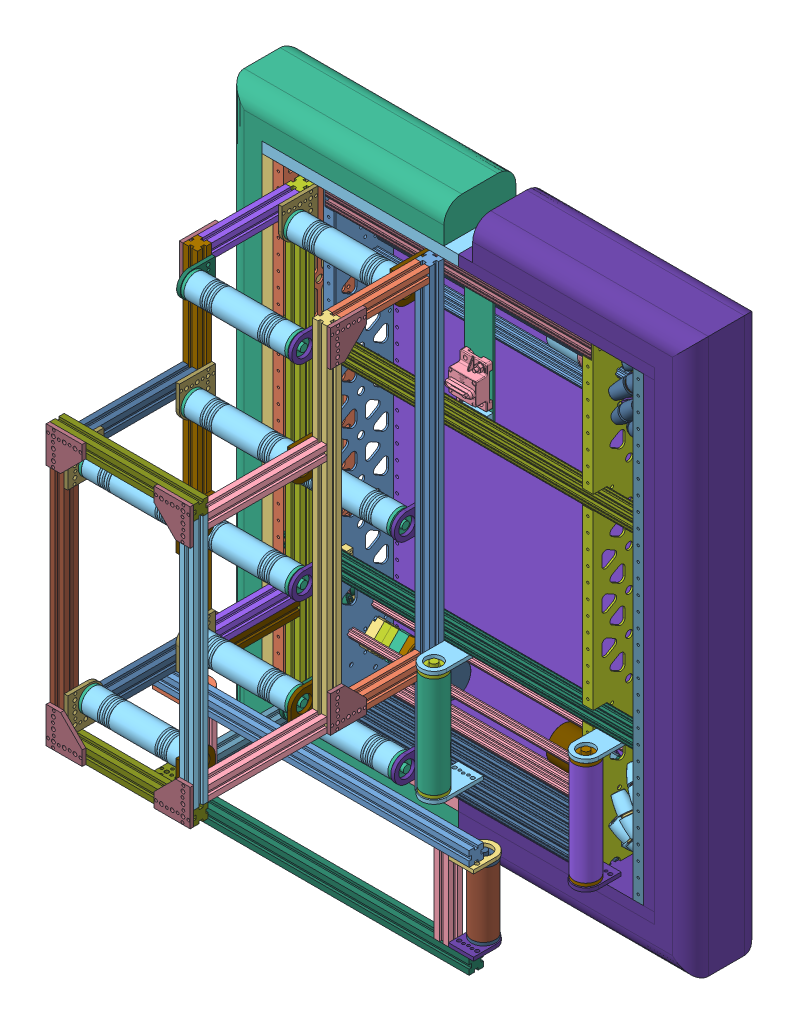
SolidWorks assembly Robot 2020, configuration Default. Lengths in mm.
Overall size (819.15 977.9 619.08).
518 component instances, 131 part files, 0 mates.
Components (placement in the parent):
- Copy of Fame 2020-1: Copy of Fame 2020 [Default] at origin size (819.15 977.9 171.99)
  - Inner plate v12(Mirror)^Copy of Fame 2020-1: Inner plate v12(Mirror)^Copy of Fame 2020 [Default] at (-212.725 0 58.7875) x (0 1 0) z (0 0 -1) size (812.8 19.05 127) (virtual)
    - Inner plate v12(Mirror)-0^Inner plate v12(Mirror)_Copy of Fame 2020-1: Inner plate v12(Mirror)-0^Inner plate v12(Mirror)_Copy of Fame 2020 [Default] at origin size (812.8 19.05 127) (virtual)
  - Outer plate v11(Mirror)^Copy of Fame 2020-1: Outer plate v11(Mirror)^Copy of Fame 2020 [Default] at (-333.375 0 58.7875) x (0 -1 0) z (0 0 -1) size (812.8 19.05 127) (virtual)
    - Outer plate v11(Mirror)-1^Outer plate v11(Mirror)_Copy of Fame 2020-1: Outer plate v11(Mirror)-1^Outer plate v11(Mirror)_Copy of Fame 2020 [Default] at origin size (812.8 19.05 127) (virtual)
  - Bumper Assembly v4(Mirror)^Copy of Fame 2020-1: Bumper Assembly v4(Mirror)^Copy of Fame 2020 [Default] at (-327.025 0.0665 58.7875) x (-1 0 0) z (0 0 -1) size (409.58 977.9 127) (virtual)
    - Bumper Assembly v4(Mirror)-2^Bumper Assembly v4(Mirror)_Copy of Fame 2020-1: Bumper Assembly v4(Mirror)-2^Bumper Assembly v4(Mirror)_Copy of Fame 2020 [Default] at origin size (19.05 812.8 127) (virtual)
    - Bumper Assembly v4(Mirror)-3^Bumper Assembly v4(Mirror)_Copy of Fame 2020-1: Bumper Assembly v4(Mirror)-3^Bumper Assembly v4(Mirror)_Copy of Fame 2020 [Default] at origin size (346.08 19.05 127) (virtual)
    - Bumper Assembly v4(Mirror)-4^Bumper Assembly v4(Mirror)_Copy of Fame 2020-1: Bumper Assembly v4(Mirror)-4^Bumper Assembly v4(Mirror)_Copy of Fame 2020 [Default] at origin size (346.08 19.05 127) (virtual)
    - Bumper Assembly v4(Mirror)-5^Bumper Assembly v4(Mirror)_Copy of Fame 2020-1: Bumper Assembly v4(Mirror)-5^Bumper Assembly v4(Mirror)_Copy of Fame 2020 [Default] at origin size (409.58 977.9 127) (virtual)
  - NEO Gearbox 2-stage Custom^Copy of Fame 2020-1: NEO Gearbox 2-stage Custom^Copy of Fame 2020 [Default] at (0 0 425) size (164.9 90.53 90.53) (virtual)
    - VersaPlanetary_4_1_Gear_Kit_217-2818^NEO Gearbox 2-stage Custom_Copy of Fame 2020-1: VersaPlanetary_4_1_Gear_Kit_217-2818^NEO Gearbox 2-stage Custom_Copy of Fame 2020 [Default] at (-15.25 22.225 0) x (0 -0.707107 0.707107) z (-1 0 0) size (35.49 35.49 17.4) (virtual)
      - 217-2725-001 Rev1_24t Sun^VersaPlanetary_4_1_Gear_Kit_217-2818_NEO Gearbox 2-stage Custom_Copy of Fame 2020-1: 217-2725-001 Rev1_24t Sun^VersaPlanetary_4_1_Gear_Kit_217-2818_NEO Gearbox 2-stage Custom_Copy of Fame 2020 [Default] at (-36.69 -517.1337 -209.675) x (0.707107 0.707107 0) z (0 0 1) size (14.4 14.45 12.7) (virtual)
      - 217-2725-002 Rev1_24t Planet^VersaPlanetary_4_1_Gear_Kit_217-2818_NEO Gearbox 2-stage Custom_Copy of Fame 2020-1: 217-2725-002 Rev1_24t Planet^VersaPlanetary_4_1_Gear_Kit_217-2818_NEO Gearbox 2-stage Custom_Copy of Fame 2020 [Default] at (-45.2382 -525.6819 -212.025) x (-0.793353 0.608761 0) z (0 0 -1) size (13.12 13.1 8) (virtual)
      - 217-2724-002 Rev1^VersaPlanetary_4_1_Gear_Kit_217-2818_NEO Gearbox 2-stage Custom_Copy of Fame 2020-1: 217-2724-002 Rev1^VersaPlanetary_4_1_Gear_Kit_217-2818_NEO Gearbox 2-stage Custom_Copy of Fame 2020 [Default] at (-36.69 -517.1337 -218.375) x (1 0 0) z (0 0 -1) size (34.7 34.7 4.7) (virtual)
      - 217-2625-010 Rev1^VersaPlanetary_4_1_Gear_Kit_217-2818_NEO Gearbox 2-stage Custom_Copy of Fame 2020-1: 217-2625-010 Rev1^VersaPlanetary_4_1_Gear_Kit_217-2818_NEO Gearbox 2-stage Custom_Copy of Fame 2020 [Default] at (-45.2382 -525.6819 -214.725) x (0.854322 0.519745 0) z (0 0 1) size (4 4 12) (virtual)
      - 217-2725-002 Rev1_24t Planet^VersaPlanetary_4_1_Gear_Kit_217-2818_NEO Gearbox 2-stage Custom_Copy of Fame 2020-2: 217-2725-002 Rev1_24t Planet^VersaPlanetary_4_1_Gear_Kit_217-2818_NEO Gearbox 2-stage Custom_Copy of Fame 2020 [Default] at (-28.1418 -525.6819 -212.025) x (-0.608761 -0.793353 0) z (0 0 -1) size (13.12 13.1 8) (virtual)
      - 217-2725-002 Rev1_24t Planet^VersaPlanetary_4_1_Gear_Kit_217-2818_NEO Gearbox 2-stage Custom_Copy of Fame 2020-3: 217-2725-002 Rev1_24t Planet^VersaPlanetary_4_1_Gear_Kit_217-2818_NEO Gearbox 2-stage Custom_Copy of Fame 2020 [Default] at (-28.1418 -508.5855 -212.025) x (0.793353 -0.608761 0) z (0 0 -1) size (13.12 13.1 8) (virtual)
      - 217-2725-002 Rev1_24t Planet^VersaPlanetary_4_1_Gear_Kit_217-2818_NEO Gearbox 2-stage Custom_Copy of Fame 2020-4: 217-2725-002 Rev1_24t Planet^VersaPlanetary_4_1_Gear_Kit_217-2818_NEO Gearbox 2-stage Custom_Copy of Fame 2020 [Default] at (-45.2382 -508.5855 -212.025) x (0.608761 0.793353 0) z (0 0 -1) size (13.12 13.1 8) (virtual)
      - 217-2625-010 Rev1^VersaPlanetary_4_1_Gear_Kit_217-2818_NEO Gearbox 2-stage Custom_Copy of Fame 2020-2: 217-2625-010 Rev1^VersaPlanetary_4_1_Gear_Kit_217-2818_NEO Gearbox 2-stage Custom_Copy of Fame 2020 [Default] at (-28.1418 -525.6819 -214.725) x (-0.519745 0.854322 0) z (0 0 1) size (4 4 12) (virtual)
      - 217-2625-010 Rev1^VersaPlanetary_4_1_Gear_Kit_217-2818_NEO Gearbox 2-stage Custom_Copy of Fame 2020-3: 217-2625-010 Rev1^VersaPlanetary_4_1_Gear_Kit_217-2818_NEO Gearbox 2-stage Custom_Copy of Fame 2020 [Default] at (-28.1418 -508.5855 -214.725) x (-0.854322 -0.519745 0) z (0 0 1) size (4 4 12) (virtual)
      - 217-2625-010 Rev1^VersaPlanetary_4_1_Gear_Kit_217-2818_NEO Gearbox 2-stage Custom_Copy of Fame 2020-4: 217-2625-010 Rev1^VersaPlanetary_4_1_Gear_Kit_217-2818_NEO Gearbox 2-stage Custom_Copy of Fame 2020 [Default] at (-45.2382 -508.5855 -214.725) x (0.519745 -0.854322 0) z (0 0 1) size (4 4 12) (virtual)
    - 217-2625-026 Rev1^NEO Gearbox 2-stage Custom_Copy of Fame 2020-1: 217-2625-026 Rev1^NEO Gearbox 2-stage Custom_Copy of Fame 2020 [Default] at (211.875 -317.5 -391.6125) x (0 -0.707107 0.707107) z (-1 0 0) size (44.45 42 18.12) (virtual)
    - 217-2742-001 Rev4^NEO Gearbox 2-stage Custom_Copy of Fame 2020-1: 217-2742-001 Rev4^NEO Gearbox 2-stage Custom_Copy of Fame 2020 [Default] at (218.5752 -317.5 -391.6125) x (1 0 0) z (0 0.63857 0.769564) size (7 28 28) (virtual)
    - 217-2742-001 Rev4^NEO Gearbox 2-stage Custom_Copy of Fame 2020-2: 217-2742-001 Rev4^NEO Gearbox 2-stage Custom_Copy of Fame 2020 [Default] at (226.5752 -317.5 -391.6125) x (1 0 0) z (0 0.707107 0.707107) size (7 28 28) (virtual)
    - 217-2625-017 Rev1_9714K61^NEO Gearbox 2-stage Custom_Copy of Fame 2020-1: 217-2625-017 Rev1_9714K61^NEO Gearbox 2-stage Custom_Copy of Fame 2020 [Default] at (225.795 -317.6887 -391.9075) x (0 0.983393 0.181491) z (0 -0.181491 0.983393) size (28.51 4.98 27.43) (virtual)
    - 217-2625-025 Rev1^NEO Gearbox 2-stage Custom_Copy of Fame 2020-1: 217-2625-025 Rev1^NEO Gearbox 2-stage Custom_Copy of Fame 2020 [Default] at (182.475 -317.5 -391.6125) x (0 -0.707107 0.707107) z (-1 0 0) size (44.45 42 18) (virtual)
    - 217-2816-001 Rev1^NEO Gearbox 2-stage Custom_Copy of Fame 2020-1: 217-2816-001 Rev1^NEO Gearbox 2-stage Custom_Copy of Fame 2020 [Default] at (212.025 -317.5 -391.6125) x (0 -0.707107 0.707107) z (1 0 0) size (42 42 14.5) (virtual)
    - 217-2816-001 Rev1^NEO Gearbox 2-stage Custom_Copy of Fame 2020-2: 217-2816-001 Rev1^NEO Gearbox 2-stage Custom_Copy of Fame 2020 [Default] at (199.325 -317.5 -391.6125) x (0 -0.707107 0.707107) z (1 0 0) size (42 42 14.5) (virtual)
    - 217-4649-001 Rev1^NEO Gearbox 2-stage Custom_Copy of Fame 2020-1: 217-4649-001 Rev1^NEO Gearbox 2-stage Custom_Copy of Fame 2020 [Default] at (185.629 -317.5 -391.6125) x (0 -0.707107 0.707107) z (1 0 0) size (18 18 13) (virtual)
    - VersaPlanetary_CIM_Adapter_217-4018^NEO Gearbox 2-stage Custom_Copy of Fame 2020-1: VersaPlanetary_CIM_Adapter_217-4018^NEO Gearbox 2-stage Custom_Copy of Fame 2020 [Default] at (165.15 -317.5 -391.6125) x (0 -0.707107 0.707107) z (0 0.707107 0.707107) size (64.01 21.55 64.01) (virtual)
    - NEO Motor REV-21-1650^NEO Gearbox 2-stage Custom_Copy of Fame 2020-1: NEO Motor REV-21-1650^NEO Gearbox 2-stage Custom_Copy of Fame 2020 [Default] at (153.625 -317.5 -391.6125) x (0 -0.707107 -0.707107) z (1 0 0) size (61.14 61.02 93.25) (virtual)
    - 3_1 Output Shaft Custom^NEO Gearbox 2-stage Custom_Copy of Fame 2020-1: 3_1 Output Shaft Custom^NEO Gearbox 2-stage Custom_Copy of Fame 2020 [Default] at (211.3752 -317.5 -391.6125) x (1 0 0) z (0 0.707107 0.707107) size (48.9 34.7 34.7) (virtual)
  - Left Wheel Assembly^Copy of Fame 2020-1: Left Wheel Assembly^Copy of Fame 2020 [Default] at (500 0 0) size (65.82 166.11 165.01) (virtual)
    - 6_Mecanum_Wheel_Left_217-2799^Left Wheel Assembly_Copy of Fame 2020-1: 6_Mecanum_Wheel_Left_217-2799^Left Wheel Assembly_Copy of Fame 2020 [Default] x (0 0 1) z (-1 0 0) size (165.01 166.11 65.82) (virtual)
      - 217-2799-001 Rev1^6_Mecanum_Wheel_Left_217-2799_Left Wheel Assembly_Copy of Fame 2020-1: 217-2799-001 Rev1^6_Mecanum_Wheel_Left_217-2799_Left Wheel Assembly_Copy of Fame 2020 [Default] at (33.3875 -317.5 234.0098) x (0.707107 0.707107 0) z (0 0 1) size (95.78 100.46 28.55) (virtual)
      - 217-2799-001 Rev1^6_Mecanum_Wheel_Left_217-2799_Left Wheel Assembly_Copy of Fame 2020-2: 217-2799-001 Rev1^6_Mecanum_Wheel_Left_217-2799_Left Wheel Assembly_Copy of Fame 2020 [Default] at (33.3875 -317.5 221.3098) x (-0.987688 -0.156434 0) z (0 0 -1) size (95.78 100.46 28.55) (virtual)
      - 217-2799-002 Rev1^6_Mecanum_Wheel_Left_217-2799_Left Wheel Assembly_Copy of Fame 2020-1: 217-2799-002 Rev1^6_Mecanum_Wheel_Left_217-2799_Left Wheel Assembly_Copy of Fame 2020 [Default] at (4.057 -346.8305 227.6598) x (-0.707107 0.707107 0) z (-0.707107 -0.707107 0) size (26.84 25.39 30.1) (virtual)
      - 217-2586-003 Rev2^6_Mecanum_Wheel_Left_217-2799_Left Wheel Assembly_Copy of Fame 2020-1: 217-2586-003 Rev2^6_Mecanum_Wheel_Left_217-2799_Left Wheel Assembly_Copy of Fame 2020 [Default] at (-13.4676 -358.6894 223.6536) x (0.41944 0.854155 0.30739) z (-0.757674 0.142894 0.636798) size (19.46 28.57 19.46) (virtual)
      - 217-2586-003 Rev2^6_Mecanum_Wheel_Left_217-2799_Left Wheel Assembly_Copy of Fame 2020-2: 217-2586-003 Rev2^6_Mecanum_Wheel_Left_217-2799_Left Wheel Assembly_Copy of Fame 2020 [Default] at (-7.8019 -364.3551 231.666) x (0.847342 0.451134 -0.280161) z (0.17892 -0.739241 -0.649238) size (19.46 28.57 19.46) (virtual)
      - 217-2586-004 Rev1^6_Mecanum_Wheel_Left_217-2799_Left Wheel Assembly_Copy of Fame 2020-1: 217-2586-004 Rev1^6_Mecanum_Wheel_Left_217-2799_Left Wheel Assembly_Copy of Fame 2020 [Default] at (-10.3479 -361.809 228.0654) x (-0.690521 -0.722949 -0.02293) z (0.522667 -0.476807 -0.706735) size (25.9 28.58 25.9) (virtual)
      - 217-2586-004 Rev1^6_Mecanum_Wheel_Left_217-2799_Left Wheel Assembly_Copy of Fame 2020-2: 217-2586-004 Rev1^6_Mecanum_Wheel_Left_217-2799_Left Wheel Assembly_Copy of Fame 2020 [Default] at (-10.9209 -361.2361 227.2551) x (0.01458 -0.811521 -0.584142) z (-0.865903 -0.302381 0.39847) size (25.9 28.58 25.9) (virtual)
      - 217-2586-007 Rev1^6_Mecanum_Wheel_Left_217-2799_Left Wheel Assembly_Copy of Fame 2020-1: 217-2586-007 Rev1^6_Mecanum_Wheel_Left_217-2799_Left Wheel Assembly_Copy of Fame 2020 [Default] at (-10.6347 -361.5222 227.6598) x (0.5 -0.5 0.707107) z (-0.709055 -0.705148 0.002763) size (61.72 5 5) (virtual)
      - 217-2586-008 Rev1^6_Mecanum_Wheel_Left_217-2799_Left Wheel Assembly_Copy of Fame 2020-1: 217-2586-008 Rev1^6_Mecanum_Wheel_Left_217-2799_Left Wheel Assembly_Copy of Fame 2020 [Default] at (53.3583 -330.4692 227.5328) x (0.544639 0.838671 0) z (0 0 -1) size (7.33 6.35 31.75) (virtual)
      - NUT-832-NYLOCK^6_Mecanum_Wheel_Left_217-2799_Left Wheel Assembly_Copy of Fame 2020-1: NUT-832-NYLOCK^6_Mecanum_Wheel_Left_217-2799_Left Wheel Assembly_Copy of Fame 2020 [Default] at (6.1639 -290.2764 241.3161) x (0.258819 -0.965926 0) z (-0.965926 -0.258819 0) size (9.37 5.86 8.12) (virtual)
      - SCREW-832-1250^6_Mecanum_Wheel_Left_217-2799_Left Wheel Assembly_Copy of Fame 2020-1: SCREW-832-1250^6_Mecanum_Wheel_Left_217-2799_Left Wheel Assembly_Copy of Fame 2020 [Default] at (6.1639 -290.2764 212.75) x (0 0 1) z (-0.394243 0.919006 0) size (33.96 7.92 7.92) (virtual)
      - 217-2586-007 Rev1^6_Mecanum_Wheel_Left_217-2799_Left Wheel Assembly_Copy of Fame 2020-2: 217-2586-007 Rev1^6_Mecanum_Wheel_Left_217-2799_Left Wheel Assembly_Copy of Fame 2020 [Default] at (-28.1029 -327.2391 227.6598) x (0.110616 -0.698401 0.707107) z (-0.988113 -0.153705 0.002763) size (61.72 5 5) (virtual)
      - 217-2586-007 Rev1^6_Mecanum_Wheel_Left_217-2799_Left Wheel Assembly_Copy of Fame 2020-3: 217-2586-007 Rev1^6_Mecanum_Wheel_Left_217-2799_Left Wheel Assembly_Copy of Fame 2020 [Default] at (-22.0838 -289.236 227.6598) x (-0.32102 -0.630037 0.707107) z (-0.889746 0.456448 0.002763) size (61.72 5 5) (virtual)
      - 217-2586-007 Rev1^6_Mecanum_Wheel_Left_217-2799_Left Wheel Assembly_Copy of Fame 2020-4: 217-2586-007 Rev1^6_Mecanum_Wheel_Left_217-2799_Left Wheel Assembly_Copy of Fame 2020 [Default] at (5.1235 -262.0287 227.6598) x (-0.630037 -0.32102 0.707107) z (-0.451526 0.892254 0.002763) size (61.72 5 5) (virtual)
      - 217-2586-007 Rev1^6_Mecanum_Wheel_Left_217-2799_Left Wheel Assembly_Copy of Fame 2020-5: 217-2586-007 Rev1^6_Mecanum_Wheel_Left_217-2799_Left Wheel Assembly_Copy of Fame 2020 [Default] at (43.1266 -256.0096 227.6598) x (-0.698401 0.110616 0.707107) z (0.159162 0.987249 0.002763) size (61.72 5 5) (virtual)
      - 217-2586-007 Rev1^6_Mecanum_Wheel_Left_217-2799_Left Wheel Assembly_Copy of Fame 2020-6: 217-2586-007 Rev1^6_Mecanum_Wheel_Left_217-2799_Left Wheel Assembly_Copy of Fame 2020 [Default] at (77.4097 -273.4778 227.6598) x (-0.5 0.5 0.707107) z (0.709055 0.705148 0.002763) size (61.72 5 5) (virtual)
      - 217-2586-007 Rev1^6_Mecanum_Wheel_Left_217-2799_Left Wheel Assembly_Copy of Fame 2020-7: 217-2586-007 Rev1^6_Mecanum_Wheel_Left_217-2799_Left Wheel Assembly_Copy of Fame 2020 [Default] at (94.8779 -307.7609 227.6598) x (-0.110616 0.698401 0.707107) z (0.988113 0.153705 0.002763) size (61.72 5 5) (virtual)
      - 217-2586-007 Rev1^6_Mecanum_Wheel_Left_217-2799_Left Wheel Assembly_Copy of Fame 2020-8: 217-2586-007 Rev1^6_Mecanum_Wheel_Left_217-2799_Left Wheel Assembly_Copy of Fame 2020 [Default] at (88.8588 -345.764 227.6598) x (0.32102 0.630037 0.707107) z (0.889746 -0.456448 0.002763) size (61.72 5 5) (virtual)
      - 217-2586-007 Rev1^6_Mecanum_Wheel_Left_217-2799_Left Wheel Assembly_Copy of Fame 2020-9: 217-2586-007 Rev1^6_Mecanum_Wheel_Left_217-2799_Left Wheel Assembly_Copy of Fame 2020 [Default] at (61.6515 -372.9713 227.6598) x (0.630037 0.32102 0.707107) z (0.451526 -0.892254 0.002763) size (61.72 5 5) (virtual)
      - 217-2586-007 Rev1^6_Mecanum_Wheel_Left_217-2799_Left Wheel Assembly_Copy of Fame 2020-10: 217-2586-007 Rev1^6_Mecanum_Wheel_Left_217-2799_Left Wheel Assembly_Copy of Fame 2020 [Default] at (23.6484 -378.9904 227.6598) x (0.698401 -0.110616 0.707107) z (-0.159162 -0.987249 0.002763) size (61.72 5 5) (virtual)
      - 217-2586-004 Rev1^6_Mecanum_Wheel_Left_217-2799_Left Wheel Assembly_Copy of Fame 2020-3: 217-2586-004 Rev1^6_Mecanum_Wheel_Left_217-2799_Left Wheel Assembly_Copy of Fame 2020 [Default] at (-28.1662 -326.8394 227.2551) x (-0.465204 -0.665104 -0.584142) z (-0.878265 0.264334 0.39847) size (25.9 28.58 25.9) (virtual)
      - 217-2586-004 Rev1^6_Mecanum_Wheel_Left_217-2799_Left Wheel Assembly_Copy of Fame 2020-4: 217-2586-004 Rev1^6_Mecanum_Wheel_Left_217-2799_Left Wheel Assembly_Copy of Fame 2020 [Default] at (-21.9 -288.8754 227.2551) x (-0.767297 -0.26464 -0.584142) z (-0.55516 0.730082 0.39847) size (25.9 28.58 25.9) (virtual)
      - 217-2586-004 Rev1^6_Mecanum_Wheel_Left_217-2799_Left Wheel Assembly_Copy of Fame 2020-5: 217-2586-004 Rev1^6_Mecanum_Wheel_Left_217-2799_Left Wheel Assembly_Copy of Fame 2020 [Default] at (5.484 -261.845 227.2551) x (-0.776308 0.236907 -0.584142) z (-0.020002 0.916963 0.39847) size (25.9 28.58 25.9) (virtual)
      - 217-2586-004 Rev1^6_Mecanum_Wheel_Left_217-2799_Left Wheel Assembly_Copy of Fame 2020-6: 217-2586-004 Rev1^6_Mecanum_Wheel_Left_217-2799_Left Wheel Assembly_Copy of Fame 2020 [Default] at (43.5263 -256.0729 227.2551) x (-0.488796 0.647964 -0.584142) z (0.522795 0.753596 0.39847) size (25.9 28.58 25.9) (virtual)
      - 217-2586-004 Rev1^6_Mecanum_Wheel_Left_217-2799_Left Wheel Assembly_Copy of Fame 2020-7: 217-2586-004 Rev1^6_Mecanum_Wheel_Left_217-2799_Left Wheel Assembly_Copy of Fame 2020 [Default] at (77.6959 -273.7639 227.2551) x (-0.01458 0.811521 -0.584142) z (0.865903 0.302381 0.39847) size (25.9 28.58 25.9) (virtual)
      - 217-2586-004 Rev1^6_Mecanum_Wheel_Left_217-2799_Left Wheel Assembly_Copy of Fame 2020-8: 217-2586-004 Rev1^6_Mecanum_Wheel_Left_217-2799_Left Wheel Assembly_Copy of Fame 2020 [Default] at (94.9412 -308.1606 227.2551) x (0.465204 0.665104 -0.584142) z (0.878265 -0.264334 0.39847) size (25.9 28.58 25.9) (virtual)
      - 217-2586-004 Rev1^6_Mecanum_Wheel_Left_217-2799_Left Wheel Assembly_Copy of Fame 2020-9: 217-2586-004 Rev1^6_Mecanum_Wheel_Left_217-2799_Left Wheel Assembly_Copy of Fame 2020 [Default] at (88.675 -346.1246 227.2551) x (0.767297 0.26464 -0.584142) z (0.55516 -0.730082 0.39847) size (25.9 28.58 25.9) (virtual)
      - 217-2586-004 Rev1^6_Mecanum_Wheel_Left_217-2799_Left Wheel Assembly_Copy of Fame 2020-10: 217-2586-004 Rev1^6_Mecanum_Wheel_Left_217-2799_Left Wheel Assembly_Copy of Fame 2020 [Default] at (61.291 -373.155 227.2551) x (0.776308 -0.236907 -0.584142) z (0.020002 -0.916963 0.39847) size (25.9 28.58 25.9) (virtual)
      - 217-2586-004 Rev1^6_Mecanum_Wheel_Left_217-2799_Left Wheel Assembly_Copy of Fame 2020-11: 217-2586-004 Rev1^6_Mecanum_Wheel_Left_217-2799_Left Wheel Assembly_Copy of Fame 2020 [Default] at (23.2487 -378.9271 227.2551) x (0.488796 -0.647964 -0.584142) z (-0.522795 -0.753596 0.39847) size (25.9 28.58 25.9) (virtual)
      - 217-2586-004 Rev1^6_Mecanum_Wheel_Left_217-2799_Left Wheel Assembly_Copy of Fame 2020-12: 217-2586-004 Rev1^6_Mecanum_Wheel_Left_217-2799_Left Wheel Assembly_Copy of Fame 2020 [Default] at (-28.0394 -327.6397 228.0654) x (-0.983582 -0.179 -0.02293) z (0.142587 -0.692961 -0.706735) size (25.9 28.58 25.9) (virtual)
      - 217-2586-004 Rev1^6_Mecanum_Wheel_Left_217-2799_Left Wheel Assembly_Copy of Fame 2020-13: 217-2586-004 Rev1^6_Mecanum_Wheel_Left_217-2799_Left Wheel Assembly_Copy of Fame 2020 [Default] at (-22.2679 -289.5974 228.0654) x (-0.900948 0.433321 -0.02293) z (-0.291957 -0.644427 -0.706735) size (25.9 28.58 25.9) (virtual)
      - 217-2586-004 Rev1^6_Mecanum_Wheel_Left_217-2799_Left Wheel Assembly_Copy of Fame 2020-14: 217-2586-004 Rev1^6_Mecanum_Wheel_Left_217-2799_Left Wheel Assembly_Copy of Fame 2020 [Default] at (4.7621 -262.2129 228.0654) x (-0.474183 0.880128 -0.02293) z (-0.614983 -0.349745 -0.706735) size (25.9 28.58 25.9) (virtual)
      - 217-2586-004 Rev1^6_Mecanum_Wheel_Left_217-2799_Left Wheel Assembly_Copy of Fame 2020-15: 217-2586-004 Rev1^6_Mecanum_Wheel_Left_217-2799_Left Wheel Assembly_Copy of Fame 2020 [Default] at (42.726 -255.9462 228.0654) x (0.133704 0.990756 -0.02293) z (-0.703107 0.078529 -0.706735) size (25.9 28.58 25.9) (virtual)
      - 217-2586-004 Rev1^6_Mecanum_Wheel_Left_217-2799_Left Wheel Assembly_Copy of Fame 2020-16: 217-2586-004 Rev1^6_Mecanum_Wheel_Left_217-2799_Left Wheel Assembly_Copy of Fame 2020 [Default] at (77.1229 -273.191 228.0654) x (0.690521 0.722949 -0.02293) z (-0.522667 0.476807 -0.706735) size (25.9 28.58 25.9) (virtual)
      - 217-2586-004 Rev1^6_Mecanum_Wheel_Left_217-2799_Left Wheel Assembly_Copy of Fame 2020-17: 217-2586-004 Rev1^6_Mecanum_Wheel_Left_217-2799_Left Wheel Assembly_Copy of Fame 2020 [Default] at (94.8144 -307.3603 228.0654) x (0.983582 0.179 -0.02293) z (-0.142587 0.692961 -0.706735) size (25.9 28.58 25.9) (virtual)
      - 217-2586-004 Rev1^6_Mecanum_Wheel_Left_217-2799_Left Wheel Assembly_Copy of Fame 2020-18: 217-2586-004 Rev1^6_Mecanum_Wheel_Left_217-2799_Left Wheel Assembly_Copy of Fame 2020 [Default] at (89.0429 -345.4026 228.0654) x (0.900948 -0.433321 -0.02293) z (0.291957 0.644427 -0.706735) size (25.9 28.58 25.9) (virtual)
      - 217-2586-004 Rev1^6_Mecanum_Wheel_Left_217-2799_Left Wheel Assembly_Copy of Fame 2020-19: 217-2586-004 Rev1^6_Mecanum_Wheel_Left_217-2799_Left Wheel Assembly_Copy of Fame 2020 [Default] at (62.0129 -372.7871 228.0654) x (0.474183 -0.880128 -0.02293) z (0.614983 0.349745 -0.706735) size (25.9 28.58 25.9) (virtual)
      - 217-2586-004 Rev1^6_Mecanum_Wheel_Left_217-2799_Left Wheel Assembly_Copy of Fame 2020-20: 217-2586-004 Rev1^6_Mecanum_Wheel_Left_217-2799_Left Wheel Assembly_Copy of Fame 2020 [Default] at (24.049 -379.0538 228.0654) x (-0.133704 -0.990756 -0.02293) z (0.703107 -0.078529 -0.706735) size (25.9 28.58 25.9) (virtual)
      - 217-2586-003 Rev2^6_Mecanum_Wheel_Left_217-2799_Left Wheel Assembly_Copy of Fame 2020-3: 217-2586-003 Rev2^6_Mecanum_Wheel_Left_217-2799_Left Wheel Assembly_Copy of Fame 2020 [Default] at (-27.4761 -331.196 231.666) x (0.950684 -0.13308 -0.280161) z (-0.289766 -0.703225 -0.649238) size (19.46 28.57 19.46) (virtual)
      - 217-2586-003 Rev2^6_Mecanum_Wheel_Left_217-2799_Left Wheel Assembly_Copy of Fame 2020-4: 217-2586-003 Rev2^6_Mecanum_Wheel_Left_217-2799_Left Wheel Assembly_Copy of Fame 2020 [Default] at (-23.9025 -292.8056 231.666) x (0.690897 -0.666462 -0.280161) z (-0.647771 -0.398601 -0.649238) size (19.46 28.57 19.46) (virtual)
      - 217-2586-003 Rev2^6_Mecanum_Wheel_Left_217-2799_Left Wheel Assembly_Copy of Fame 2020-5: 217-2586-003 Rev2^6_Mecanum_Wheel_Left_217-2799_Left Wheel Assembly_Copy of Fame 2020 [Default] at (1.5539 -263.8475 231.666) x (0.167211 -0.945278 -0.280161) z (-0.75835 0.058276 -0.649238) size (19.46 28.57 19.46) (virtual)
      - 217-2586-003 Rev2^6_Mecanum_Wheel_Left_217-2799_Left Wheel Assembly_Copy of Fame 2020-6: 217-2586-003 Rev2^6_Mecanum_Wheel_Left_217-2799_Left Wheel Assembly_Copy of Fame 2020 [Default] at (39.1697 -255.3829 231.666) x (-0.420344 -0.86303 -0.280161) z (-0.579264 0.492893 -0.649238) size (19.46 28.57 19.46) (virtual)
      - 217-2586-003 Rev2^6_Mecanum_Wheel_Left_217-2799_Left Wheel Assembly_Copy of Fame 2020-7: 217-2586-003 Rev2^6_Mecanum_Wheel_Left_217-2799_Left Wheel Assembly_Copy of Fame 2020 [Default] at (74.5769 -270.6449 231.666) x (-0.847342 -0.451134 -0.280161) z (-0.17892 0.739241 -0.649238) size (19.46 28.57 19.46) (virtual)
      - 217-2586-003 Rev2^6_Mecanum_Wheel_Left_217-2799_Left Wheel Assembly_Copy of Fame 2020-8: 217-2586-003 Rev2^6_Mecanum_Wheel_Left_217-2799_Left Wheel Assembly_Copy of Fame 2020 [Default] at (94.2511 -303.804 231.666) x (-0.950684 0.13308 -0.280161) z (0.289766 0.703225 -0.649238) size (19.46 28.57 19.46) (virtual)
      - 217-2586-003 Rev2^6_Mecanum_Wheel_Left_217-2799_Left Wheel Assembly_Copy of Fame 2020-9: 217-2586-003 Rev2^6_Mecanum_Wheel_Left_217-2799_Left Wheel Assembly_Copy of Fame 2020 [Default] at (90.6775 -342.1944 231.666) x (-0.690897 0.666462 -0.280161) z (0.647771 0.398601 -0.649238) size (19.46 28.57 19.46) (virtual)
      - 217-2586-003 Rev2^6_Mecanum_Wheel_Left_217-2799_Left Wheel Assembly_Copy of Fame 2020-10: 217-2586-003 Rev2^6_Mecanum_Wheel_Left_217-2799_Left Wheel Assembly_Copy of Fame 2020 [Default] at (65.2211 -371.1525 231.666) x (-0.167211 0.945278 -0.280161) z (0.75835 -0.058276 -0.649238) size (19.46 28.57 19.46) (virtual)
      - 217-2586-003 Rev2^6_Mecanum_Wheel_Left_217-2799_Left Wheel Assembly_Copy of Fame 2020-11: 217-2586-003 Rev2^6_Mecanum_Wheel_Left_217-2799_Left Wheel Assembly_Copy of Fame 2020 [Default] at (27.6053 -379.6171 231.666) x (0.420344 0.86303 -0.280161) z (0.579264 -0.492893 -0.649238) size (19.46 28.57 19.46) (virtual)
      - 217-2586-003 Rev2^6_Mecanum_Wheel_Left_217-2799_Left Wheel Assembly_Copy of Fame 2020-12: 217-2586-003 Rev2^6_Mecanum_Wheel_Left_217-2799_Left Wheel Assembly_Copy of Fame 2020 [Default] at (-28.7296 -323.2822 223.6536) x (0.841394 0.444485 0.30739) z (-0.52898 0.560953 0.636798) size (19.46 28.57 19.46) (virtual)
      - 217-2586-003 Rev2^6_Mecanum_Wheel_Left_217-2799_Left Wheel Assembly_Copy of Fame 2020-13: 217-2586-003 Rev2^6_Mecanum_Wheel_Left_217-2799_Left Wheel Assembly_Copy of Fame 2020 [Default] at (-20.265 -285.6664 223.6536) x (0.941964 -0.134963 0.30739) z (-0.098234 0.764747 0.636798) size (19.46 28.57 19.46) (virtual)
      - 217-2586-003 Rev2^6_Mecanum_Wheel_Left_217-2799_Left Wheel Assembly_Copy of Fame 2020-14: 217-2586-003 Rev2^6_Mecanum_Wheel_Left_217-2799_Left Wheel Assembly_Copy of Fame 2020 [Default] at (8.6931 -260.21 223.6536) x (0.682736 -0.66286 0.30739) z (0.370035 0.676434 0.636798) size (19.46 28.57 19.46) (virtual)
      - 217-2586-003 Rev2^6_Mecanum_Wheel_Left_217-2799_Left Wheel Assembly_Copy of Fame 2020-15: 217-2586-003 Rev2^6_Mecanum_Wheel_Left_217-2799_Left Wheel Assembly_Copy of Fame 2020 [Default] at (47.0835 -256.6364 223.6536) x (0.162726 -0.937567 0.30739) z (0.696962 0.329746 0.636798) size (19.46 28.57 19.46) (virtual)
      - 217-2586-003 Rev2^6_Mecanum_Wheel_Left_217-2799_Left Wheel Assembly_Copy of Fame 2020-16: 217-2586-003 Rev2^6_Mecanum_Wheel_Left_217-2799_Left Wheel Assembly_Copy of Fame 2020 [Default] at (80.2426 -276.3106 223.6536) x (-0.41944 -0.854155 0.30739) z (0.757674 -0.142894 0.636798) size (19.46 28.57 19.46) (virtual)
      - 217-2586-003 Rev2^6_Mecanum_Wheel_Left_217-2799_Left Wheel Assembly_Copy of Fame 2020-17: 217-2586-003 Rev2^6_Mecanum_Wheel_Left_217-2799_Left Wheel Assembly_Copy of Fame 2020 [Default] at (95.5046 -311.7178 223.6536) x (-0.841394 -0.444485 0.30739) z (0.52898 -0.560953 0.636798) size (19.46 28.57 19.46) (virtual)
      - 217-2586-003 Rev2^6_Mecanum_Wheel_Left_217-2799_Left Wheel Assembly_Copy of Fame 2020-18: 217-2586-003 Rev2^6_Mecanum_Wheel_Left_217-2799_Left Wheel Assembly_Copy of Fame 2020 [Default] at (87.04 -349.3336 223.6536) x (-0.941964 0.134963 0.30739) z (0.098234 -0.764747 0.636798) size (19.46 28.57 19.46) (virtual)
      - 217-2586-003 Rev2^6_Mecanum_Wheel_Left_217-2799_Left Wheel Assembly_Copy of Fame 2020-19: 217-2586-003 Rev2^6_Mecanum_Wheel_Left_217-2799_Left Wheel Assembly_Copy of Fame 2020 [Default] at (58.0819 -374.79 223.6536) x (-0.682736 0.66286 0.30739) z (-0.370035 -0.676434 0.636798) size (19.46 28.57 19.46) (virtual)
      - 217-2586-003 Rev2^6_Mecanum_Wheel_Left_217-2799_Left Wheel Assembly_Copy of Fame 2020-20: 217-2586-003 Rev2^6_Mecanum_Wheel_Left_217-2799_Left Wheel Assembly_Copy of Fame 2020 [Default] at (19.6915 -378.3636 223.6536) x (-0.162726 0.937567 0.30739) z (-0.696962 -0.329746 0.636798) size (19.46 28.57 19.46) (virtual)
      - 217-2799-002 Rev1^6_Mecanum_Wheel_Left_217-2799_Left Wheel Assembly_Copy of Fame 2020-2: 217-2799-002 Rev1^6_Mecanum_Wheel_Left_217-2799_Left Wheel Assembly_Copy of Fame 2020 [Default] at (-7.5815 -323.9888 227.6598) x (-0.156434 0.987688 0) z (-0.987688 -0.156434 0) size (26.84 25.39 30.1) (virtual)
      - 217-2799-002 Rev1^6_Mecanum_Wheel_Left_217-2799_Left Wheel Assembly_Copy of Fame 2020-3: 217-2799-002 Rev1^6_Mecanum_Wheel_Left_217-2799_Left Wheel Assembly_Copy of Fame 2020 [Default] at (-3.5711 -298.6686 227.6598) x (0.45399 0.891007 0) z (-0.891007 0.45399 0) size (26.84 25.39 30.1) (virtual)
      - 217-2799-002 Rev1^6_Mecanum_Wheel_Left_217-2799_Left Wheel Assembly_Copy of Fame 2020-4: 217-2799-002 Rev1^6_Mecanum_Wheel_Left_217-2799_Left Wheel Assembly_Copy of Fame 2020 [Default] at (14.5561 -280.5414 227.6598) x (0.891007 0.45399 0) z (-0.45399 0.891007 0) size (26.84 25.39 30.1) (virtual)
      - 217-2799-002 Rev1^6_Mecanum_Wheel_Left_217-2799_Left Wheel Assembly_Copy of Fame 2020-5: 217-2799-002 Rev1^6_Mecanum_Wheel_Left_217-2799_Left Wheel Assembly_Copy of Fame 2020 [Default] at (39.8763 -276.531 227.6598) x (0.987688 -0.156434 0) z (0.156434 0.987688 0) size (26.84 25.39 30.1) (virtual)
      - 217-2799-002 Rev1^6_Mecanum_Wheel_Left_217-2799_Left Wheel Assembly_Copy of Fame 2020-6: 217-2799-002 Rev1^6_Mecanum_Wheel_Left_217-2799_Left Wheel Assembly_Copy of Fame 2020 [Default] at (62.718 -288.1695 227.6598) x (0.707107 -0.707107 0) z (0.707107 0.707107 0) size (26.84 25.39 30.1) (virtual)
      - 217-2799-002 Rev1^6_Mecanum_Wheel_Left_217-2799_Left Wheel Assembly_Copy of Fame 2020-7: 217-2799-002 Rev1^6_Mecanum_Wheel_Left_217-2799_Left Wheel Assembly_Copy of Fame 2020 [Default] at (74.3565 -311.0112 227.6598) x (0.156434 -0.987688 0) z (0.987688 0.156434 0) size (26.84 25.39 30.1) (virtual)
      - 217-2799-002 Rev1^6_Mecanum_Wheel_Left_217-2799_Left Wheel Assembly_Copy of Fame 2020-8: 217-2799-002 Rev1^6_Mecanum_Wheel_Left_217-2799_Left Wheel Assembly_Copy of Fame 2020 [Default] at (70.3461 -336.3314 227.6598) x (-0.45399 -0.891007 0) z (0.891007 -0.45399 0) size (26.84 25.39 30.1) (virtual)
      - 217-2799-002 Rev1^6_Mecanum_Wheel_Left_217-2799_Left Wheel Assembly_Copy of Fame 2020-9: 217-2799-002 Rev1^6_Mecanum_Wheel_Left_217-2799_Left Wheel Assembly_Copy of Fame 2020 [Default] at (52.2189 -354.4586 227.6598) x (-0.891007 -0.45399 0) z (0.45399 -0.891007 0) size (26.84 25.39 30.1) (virtual)
      - 217-2799-002 Rev1^6_Mecanum_Wheel_Left_217-2799_Left Wheel Assembly_Copy of Fame 2020-10: 217-2799-002 Rev1^6_Mecanum_Wheel_Left_217-2799_Left Wheel Assembly_Copy of Fame 2020 [Default] at (26.8987 -358.469 227.6598) x (-0.987688 0.156434 0) z (-0.156434 -0.987688 0) size (26.84 25.39 30.1) (virtual)
      - 217-2586-008 Rev1^6_Mecanum_Wheel_Left_217-2799_Left Wheel Assembly_Copy of Fame 2020-2: 217-2586-008 Rev1^6_Mecanum_Wheel_Left_217-2799_Left Wheel Assembly_Copy of Fame 2020 [Default] at (32.1413 -341.2799 227.5328) x (0.99863 -0.052336 0) z (0 0 -1) size (7.33 6.35 31.75) (virtual)
      - 217-2586-008 Rev1^6_Mecanum_Wheel_Left_217-2799_Left Wheel Assembly_Copy of Fame 2020-3: 217-2586-008 Rev1^6_Mecanum_Wheel_Left_217-2799_Left Wheel Assembly_Copy of Fame 2020 [Default] at (12.1704 -328.3106 227.5328) x (0.45399 -0.891007 0) z (0 0 -1) size (7.33 6.35 31.75) (virtual)
      - 217-2586-008 Rev1^6_Mecanum_Wheel_Left_217-2799_Left Wheel Assembly_Copy of Fame 2020-4: 217-2586-008 Rev1^6_Mecanum_Wheel_Left_217-2799_Left Wheel Assembly_Copy of Fame 2020 [Default] at (13.4167 -304.5308 227.5328) x (-0.544639 -0.838671 0) z (0 0 -1) size (7.33 6.35 31.75) (virtual)
      - 217-2586-008 Rev1^6_Mecanum_Wheel_Left_217-2799_Left Wheel Assembly_Copy of Fame 2020-5: 217-2586-008 Rev1^6_Mecanum_Wheel_Left_217-2799_Left Wheel Assembly_Copy of Fame 2020 [Default] at (34.6337 -293.7201 227.5328) x (-0.99863 0.052336 0) z (0 0 -1) size (7.33 6.35 31.75) (virtual)
      - 217-2586-008 Rev1^6_Mecanum_Wheel_Left_217-2799_Left Wheel Assembly_Copy of Fame 2020-6: 217-2586-008 Rev1^6_Mecanum_Wheel_Left_217-2799_Left Wheel Assembly_Copy of Fame 2020 [Default] at (54.6046 -306.6894 227.5328) x (-0.45399 0.891007 0) z (0 0 -1) size (7.33 6.35 31.75) (virtual)
      - SCREW-832-1250^6_Mecanum_Wheel_Left_217-2799_Left Wheel Assembly_Copy of Fame 2020-2: SCREW-832-1250^6_Mecanum_Wheel_Left_217-2799_Left Wheel Assembly_Copy of Fame 2020 [Default] at (-0.9163 -334.9786 212.75) x (0 0 1) z (-0.995855 -0.090959 0) size (33.96 7.92 7.92) (virtual)
      - SCREW-832-1250^6_Mecanum_Wheel_Left_217-2799_Left Wheel Assembly_Copy of Fame 2020-3: SCREW-832-1250^6_Mecanum_Wheel_Left_217-2799_Left Wheel Assembly_Copy of Fame 2020 [Default] at (39.4102 -355.526 212.75) x (0 0 1) z (-0.221229 -0.975222 0) size (33.96 7.92 7.92) (virtual)
      - SCREW-832-1250^6_Mecanum_Wheel_Left_217-2799_Left Wheel Assembly_Copy of Fame 2020-4: SCREW-832-1250^6_Mecanum_Wheel_Left_217-2799_Left Wheel Assembly_Copy of Fame 2020 [Default] at (71.4135 -323.5227 212.75) x (0 0 1) z (0.859128 -0.511761 0) size (33.96 7.92 7.92) (virtual)
      - SCREW-832-1250^6_Mecanum_Wheel_Left_217-2799_Left Wheel Assembly_Copy of Fame 2020-5: SCREW-832-1250^6_Mecanum_Wheel_Left_217-2799_Left Wheel Assembly_Copy of Fame 2020 [Default] at (50.8661 -283.1962 212.75) x (0 0 1) z (0.752199 0.658936 0) size (33.96 7.92 7.92) (virtual)
      - NUT-832-NYLOCK^6_Mecanum_Wheel_Left_217-2799_Left Wheel Assembly_Copy of Fame 2020-2: NUT-832-NYLOCK^6_Mecanum_Wheel_Left_217-2799_Left Wheel Assembly_Copy of Fame 2020 [Default] at (-0.9163 -334.9786 241.3161) x (0.99863 -0.052336 0) z (-0.052336 -0.99863 0) size (9.37 5.86 8.12) (virtual)
      - NUT-832-NYLOCK^6_Mecanum_Wheel_Left_217-2799_Left Wheel Assembly_Copy of Fame 2020-3: NUT-832-NYLOCK^6_Mecanum_Wheel_Left_217-2799_Left Wheel Assembly_Copy of Fame 2020 [Default] at (39.4102 -355.526 241.3161) x (0.358368 0.93358 0) z (0.93358 -0.358368 0) size (9.37 5.86 8.12) (virtual)
      - NUT-832-NYLOCK^6_Mecanum_Wheel_Left_217-2799_Left Wheel Assembly_Copy of Fame 2020-4: NUT-832-NYLOCK^6_Mecanum_Wheel_Left_217-2799_Left Wheel Assembly_Copy of Fame 2020 [Default] at (71.4135 -323.5227 241.3161) x (-0.777146 0.62932 0) z (0.62932 0.777146 0) size (9.37 5.86 8.12) (virtual)
      - NUT-832-NYLOCK^6_Mecanum_Wheel_Left_217-2799_Left Wheel Assembly_Copy of Fame 2020-5: NUT-832-NYLOCK^6_Mecanum_Wheel_Left_217-2799_Left Wheel Assembly_Copy of Fame 2020 [Default] at (50.8661 -283.1962 241.3161) x (-0.838671 -0.544639 0) z (-0.544639 0.838671 0) size (9.37 5.86 8.12) (virtual)
      - 217-2586-005 Rev2^6_Mecanum_Wheel_Left_217-2799_Left Wheel Assembly_Copy of Fame 2020-1: 217-2586-005 Rev2^6_Mecanum_Wheel_Left_217-2799_Left Wheel Assembly_Copy of Fame 2020 [Default] at (-6.1597 -365.9972 233.9884) x (-0.5 0.5 -0.707107) z (0.146447 0.853553 0.5) size (8.5 8 8) (virtual)
      - 217-2586-005 Rev2^6_Mecanum_Wheel_Left_217-2799_Left Wheel Assembly_Copy of Fame 2020-2: 217-2586-005 Rev2^6_Mecanum_Wheel_Left_217-2799_Left Wheel Assembly_Copy of Fame 2020 [Default] at (-15.1097 -357.0472 221.3312) x (-0.5 0.5 -0.707107) z (0.146447 0.853553 0.5) size (8.5 8 8) (virtual)
      - 217-2586-005 Rev2^6_Mecanum_Wheel_Left_217-2799_Left Wheel Assembly_Copy of Fame 2020-3: 217-2586-005 Rev2^6_Mecanum_Wheel_Left_217-2799_Left Wheel Assembly_Copy of Fame 2020 [Default] at (-29.0929 -320.9884 221.3312) x (-0.110616 0.698401 -0.707107) z (0.620184 0.60446 0.5) size (8.5 8 8) (virtual)
      - 217-2586-005 Rev2^6_Mecanum_Wheel_Left_217-2799_Left Wheel Assembly_Copy of Fame 2020-4: 217-2586-005 Rev2^6_Mecanum_Wheel_Left_217-2799_Left Wheel Assembly_Copy of Fame 2020 [Default] at (-19.2106 -283.5972 221.3312) x (0.32102 0.630037 -0.707107) z (0.857032 0.124484 0.5) size (8.5 8 8) (virtual)
      - 217-2586-005 Rev2^6_Mecanum_Wheel_Left_217-2799_Left Wheel Assembly_Copy of Fame 2020-5: 217-2586-005 Rev2^6_Mecanum_Wheel_Left_217-2799_Left Wheel Assembly_Copy of Fame 2020 [Default] at (10.7623 -259.1556 221.3312) x (0.630037 0.32102 -0.707107) z (0.766523 -0.403042 0.5) size (8.5 8 8) (virtual)
      - 217-2586-005 Rev2^6_Mecanum_Wheel_Left_217-2799_Left Wheel Assembly_Copy of Fame 2020-6: 217-2586-005 Rev2^6_Mecanum_Wheel_Left_217-2799_Left Wheel Assembly_Copy of Fame 2020 [Default] at (49.3773 -256.9997 221.3312) x (0.698401 -0.110616 -0.707107) z (0.383228 -0.776618 0.5) size (8.5 8 8) (virtual)
      - 217-2586-005 Rev2^6_Mecanum_Wheel_Left_217-2799_Left Wheel Assembly_Copy of Fame 2020-7: 217-2586-005 Rev2^6_Mecanum_Wheel_Left_217-2799_Left Wheel Assembly_Copy of Fame 2020 [Default] at (81.8847 -277.9528 221.3312) x (0.5 -0.5 -0.707107) z (-0.146447 -0.853553 0.5) size (8.5 8 8) (virtual)
      - 217-2586-005 Rev2^6_Mecanum_Wheel_Left_217-2799_Left Wheel Assembly_Copy of Fame 2020-8: 217-2586-005 Rev2^6_Mecanum_Wheel_Left_217-2799_Left Wheel Assembly_Copy of Fame 2020 [Default] at (95.8679 -314.0116 221.3312) x (0.110616 -0.698401 -0.707107) z (-0.620184 -0.60446 0.5) size (8.5 8 8) (virtual)
      - 217-2586-005 Rev2^6_Mecanum_Wheel_Left_217-2799_Left Wheel Assembly_Copy of Fame 2020-9: 217-2586-005 Rev2^6_Mecanum_Wheel_Left_217-2799_Left Wheel Assembly_Copy of Fame 2020 [Default] at (85.9856 -351.4028 221.3312) x (-0.32102 -0.630037 -0.707107) z (-0.857032 -0.124484 0.5) size (8.5 8 8) (virtual)
      - 217-2586-005 Rev2^6_Mecanum_Wheel_Left_217-2799_Left Wheel Assembly_Copy of Fame 2020-10: 217-2586-005 Rev2^6_Mecanum_Wheel_Left_217-2799_Left Wheel Assembly_Copy of Fame 2020 [Default] at (56.0127 -375.8444 221.3312) x (-0.630037 -0.32102 -0.707107) z (-0.766523 0.403042 0.5) size (8.5 8 8) (virtual)
      - 217-2586-005 Rev2^6_Mecanum_Wheel_Left_217-2799_Left Wheel Assembly_Copy of Fame 2020-11: 217-2586-005 Rev2^6_Mecanum_Wheel_Left_217-2799_Left Wheel Assembly_Copy of Fame 2020 [Default] at (17.3977 -378.0003 221.3312) x (-0.698401 0.110616 -0.707107) z (-0.383228 0.776618 0.5) size (8.5 8 8) (virtual)
      - 217-2586-005 Rev2^6_Mecanum_Wheel_Left_217-2799_Left Wheel Assembly_Copy of Fame 2020-12: 217-2586-005 Rev2^6_Mecanum_Wheel_Left_217-2799_Left Wheel Assembly_Copy of Fame 2020 [Default] at (-27.1128 -333.4898 233.9884) x (-0.110616 0.698401 -0.707107) z (0.620184 0.60446 0.5) size (8.5 8 8) (virtual)
      - 217-2586-005 Rev2^6_Mecanum_Wheel_Left_217-2799_Left Wheel Assembly_Copy of Fame 2020-13: 217-2586-005 Rev2^6_Mecanum_Wheel_Left_217-2799_Left Wheel Assembly_Copy of Fame 2020 [Default] at (-24.9569 -294.8748 233.9884) x (0.32102 0.630037 -0.707107) z (0.857032 0.124484 0.5) size (8.5 8 8) (virtual)
      - 217-2586-005 Rev2^6_Mecanum_Wheel_Left_217-2799_Left Wheel Assembly_Copy of Fame 2020-14: 217-2586-005 Rev2^6_Mecanum_Wheel_Left_217-2799_Left Wheel Assembly_Copy of Fame 2020 [Default] at (-0.5153 -264.9019 233.9884) x (0.630037 0.32102 -0.707107) z (0.766523 -0.403042 0.5) size (8.5 8 8) (virtual)
      - 217-2586-005 Rev2^6_Mecanum_Wheel_Left_217-2799_Left Wheel Assembly_Copy of Fame 2020-15: 217-2586-005 Rev2^6_Mecanum_Wheel_Left_217-2799_Left Wheel Assembly_Copy of Fame 2020 [Default] at (36.8759 -255.0196 233.9884) x (0.698401 -0.110616 -0.707107) z (0.383228 -0.776618 0.5) size (8.5 8 8) (virtual)
      - 217-2586-005 Rev2^6_Mecanum_Wheel_Left_217-2799_Left Wheel Assembly_Copy of Fame 2020-16: 217-2586-005 Rev2^6_Mecanum_Wheel_Left_217-2799_Left Wheel Assembly_Copy of Fame 2020 [Default] at (72.9347 -269.0028 233.9884) x (0.5 -0.5 -0.707107) z (-0.146447 -0.853553 0.5) size (8.5 8 8) (virtual)
      - 217-2586-005 Rev2^6_Mecanum_Wheel_Left_217-2799_Left Wheel Assembly_Copy of Fame 2020-17: 217-2586-005 Rev2^6_Mecanum_Wheel_Left_217-2799_Left Wheel Assembly_Copy of Fame 2020 [Default] at (93.8878 -301.5102 233.9884) x (0.110616 -0.698401 -0.707107) z (-0.620184 -0.60446 0.5) size (8.5 8 8) (virtual)
      - 217-2586-005 Rev2^6_Mecanum_Wheel_Left_217-2799_Left Wheel Assembly_Copy of Fame 2020-18: 217-2586-005 Rev2^6_Mecanum_Wheel_Left_217-2799_Left Wheel Assembly_Copy of Fame 2020 [Default] at (91.7319 -340.1252 233.9884) x (-0.32102 -0.630037 -0.707107) z (-0.857032 -0.124484 0.5) size (8.5 8 8) (virtual)
      - 217-2586-005 Rev2^6_Mecanum_Wheel_Left_217-2799_Left Wheel Assembly_Copy of Fame 2020-19: 217-2586-005 Rev2^6_Mecanum_Wheel_Left_217-2799_Left Wheel Assembly_Copy of Fame 2020 [Default] at (67.2903 -370.0981 233.9884) x (-0.630037 -0.32102 -0.707107) z (-0.766523 0.403042 0.5) size (8.5 8 8) (virtual)
      - 217-2586-005 Rev2^6_Mecanum_Wheel_Left_217-2799_Left Wheel Assembly_Copy of Fame 2020-20: 217-2586-005 Rev2^6_Mecanum_Wheel_Left_217-2799_Left Wheel Assembly_Copy of Fame 2020 [Default] at (29.8991 -379.9804 233.9884) x (-0.698401 0.110616 -0.707107) z (-0.383228 0.776618 0.5) size (8.5 8 8) (virtual)
    - 1_2_Hex_Bore_Aluminum_VersaHub_217-2592^Left Wheel Assembly_Copy of Fame 2020-1: 1_2_Hex_Bore_Aluminum_VersaHub_217-2592^Left Wheel Assembly_Copy of Fame 2020 [Default] at (-239.7248 -317.5 33.3875) x (-1 0 0) z (0 0.707107 0.707107) size (12.7 55.88 55.88) (virtual)
  - NEO Gearbox 2-stage Custom v5(Mirror) (2)^Copy of Fame 2020-1: NEO Gearbox 2-stage Custom v5(Mirror) (2)^Copy of Fame 2020 [Default] at (0 0 425) x (1 0 0) z (0 0 -1) size (164.9 90.53 90.53) (virtual)
    - VersaPlanetary_4_1_Gear_Kit_217-2818 v1(Mirror) (2)^NEO Gearbox 2-stage Custom v5(Mirror) (2)_Copy of Fame 2020-1: VersaPlanetary_4_1_Gear_Kit_217-2818 v1(Mirror) (2)^NEO Gearbox 2-stage Custom v5(Mirror) (2)_Copy of Fame 2020 [Default] at (-15.25 22.225 0) x (0 -0.707107 -0.707107) z (1 0 0) size (35.49 35.49 17.4) (virtual)
      - 217-2725-001 Rev1_24t Sun(Mirror) (2)^VersaPlanetary_4_1_Gear_Kit_217-2818 v1(Mirror) (2)_NEO Gearbox 2-stage Custom v5(Mirror) (2)_Copy of Fame 2020-1: 217-2725-001 Rev1_24t Sun(Mirror) (2)^VersaPlanetary_4_1_Gear_Kit_217-2818 v1(Mirror) (2)_NEO Gearbox 2-stage Custom v5(Mirror) (2)_Copy of Fame 2020 [Default] at (-36.69 -517.1337 209.675) x (0.707107 0.707107 0) z (0 0 1) size (14.4 14.45 12.7) (virtual)
      - 217-2725-002 Rev1_24t Planet(Mirror) (2)^VersaPlanetary_4_1_Gear_Kit_217-2818 v1(Mirror) (2)_NEO Gearbox 2-stage Custom v5(Mirror) (2)_Copy of Fame 2020-1: 217-2725-002 Rev1_24t Planet(Mirror) (2)^VersaPlanetary_4_1_Gear_Kit_217-2818 v1(Mirror) (2)_NEO Gearbox 2-stage Custom v5(Mirror) (2)_Copy of Fame 2020 [Default] at (-45.2382 -525.6819 212.025) x (-0.793353 0.608761 0) z (0 0 -1) size (13.12 13.1 8) (virtual)
      - 217-2725-002 Rev1_24t Planet(Mirror) (2)^VersaPlanetary_4_1_Gear_Kit_217-2818 v1(Mirror) (2)_NEO Gearbox 2-stage Custom v5(Mirror) (2)_Copy of Fame 2020-2: 217-2725-002 Rev1_24t Planet(Mirror) (2)^VersaPlanetary_4_1_Gear_Kit_217-2818 v1(Mirror) (2)_NEO Gearbox 2-stage Custom v5(Mirror) (2)_Copy of Fame 2020 [Default] at (-28.1418 -525.6819 212.025) x (-0.608761 -0.793353 0) z (0 0 -1) size (13.12 13.1 8) (virtual)
      - 217-2725-002 Rev1_24t Planet(Mirror) (2)^VersaPlanetary_4_1_Gear_Kit_217-2818 v1(Mirror) (2)_NEO Gearbox 2-stage Custom v5(Mirror) (2)_Copy of Fame 2020-3: 217-2725-002 Rev1_24t Planet(Mirror) (2)^VersaPlanetary_4_1_Gear_Kit_217-2818 v1(Mirror) (2)_NEO Gearbox 2-stage Custom v5(Mirror) (2)_Copy of Fame 2020 [Default] at (-28.1418 -508.5855 212.025) x (0.793353 -0.608761 0) z (0 0 -1) size (13.12 13.1 8) (virtual)
      - 217-2725-002 Rev1_24t Planet(Mirror) (2)^VersaPlanetary_4_1_Gear_Kit_217-2818 v1(Mirror) (2)_NEO Gearbox 2-stage Custom v5(Mirror) (2)_Copy of Fame 2020-4: 217-2725-002 Rev1_24t Planet(Mirror) (2)^VersaPlanetary_4_1_Gear_Kit_217-2818 v1(Mirror) (2)_NEO Gearbox 2-stage Custom v5(Mirror) (2)_Copy of Fame 2020 [Default] at (-45.2382 -508.5855 212.025) x (0.608761 0.793353 0) z (0 0 -1) size (13.12 13.1 8) (virtual)
      - 217-2724-002 Rev1(Mirror) (2)^VersaPlanetary_4_1_Gear_Kit_217-2818 v1(Mirror) (2)_NEO Gearbox 2-stage Custom v5(Mirror) (2)_Copy of Fame 2020-1: 217-2724-002 Rev1(Mirror) (2)^VersaPlanetary_4_1_Gear_Kit_217-2818 v1(Mirror) (2)_NEO Gearbox 2-stage Custom v5(Mirror) (2)_Copy of Fame 2020 [Default] at (-36.69 -517.1337 218.375) x (1 0 0) z (0 0 -1) size (34.7 34.7 4.7) (virtual)
      - 217-2625-010 Rev1(Mirror) (2)^VersaPlanetary_4_1_Gear_Kit_217-2818 v1(Mirror) (2)_NEO Gearbox 2-stage Custom v5(Mirror) (2)_Copy of Fame 2020-1: 217-2625-010 Rev1(Mirror) (2)^VersaPlanetary_4_1_Gear_Kit_217-2818 v1(Mirror) (2)_NEO Gearbox 2-stage Custom v5(Mirror) (2)_Copy of Fame 2020 [Default] at (-45.2382 -525.6819 214.725) x (0.854322 0.519745 0) z (0 0 1) size (4 4 12) (virtual)
      - 217-2625-010 Rev1(Mirror) (2)^VersaPlanetary_4_1_Gear_Kit_217-2818 v1(Mirror) (2)_NEO Gearbox 2-stage Custom v5(Mirror) (2)_Copy of Fame 2020-2: 217-2625-010 Rev1(Mirror) (2)^VersaPlanetary_4_1_Gear_Kit_217-2818 v1(Mirror) (2)_NEO Gearbox 2-stage Custom v5(Mirror) (2)_Copy of Fame 2020 [Default] at (-28.1418 -525.6819 214.725) x (-0.519745 0.854322 0) z (0 0 1) size (4 4 12) (virtual)
      - 217-2625-010 Rev1(Mirror) (2)^VersaPlanetary_4_1_Gear_Kit_217-2818 v1(Mirror) (2)_NEO Gearbox 2-stage Custom v5(Mirror) (2)_Copy of Fame 2020-3: 217-2625-010 Rev1(Mirror) (2)^VersaPlanetary_4_1_Gear_Kit_217-2818 v1(Mirror) (2)_NEO Gearbox 2-stage Custom v5(Mirror) (2)_Copy of Fame 2020 [Default] at (-28.1418 -508.5855 214.725) x (-0.854322 -0.519745 0) z (0 0 1) size (4 4 12) (virtual)
